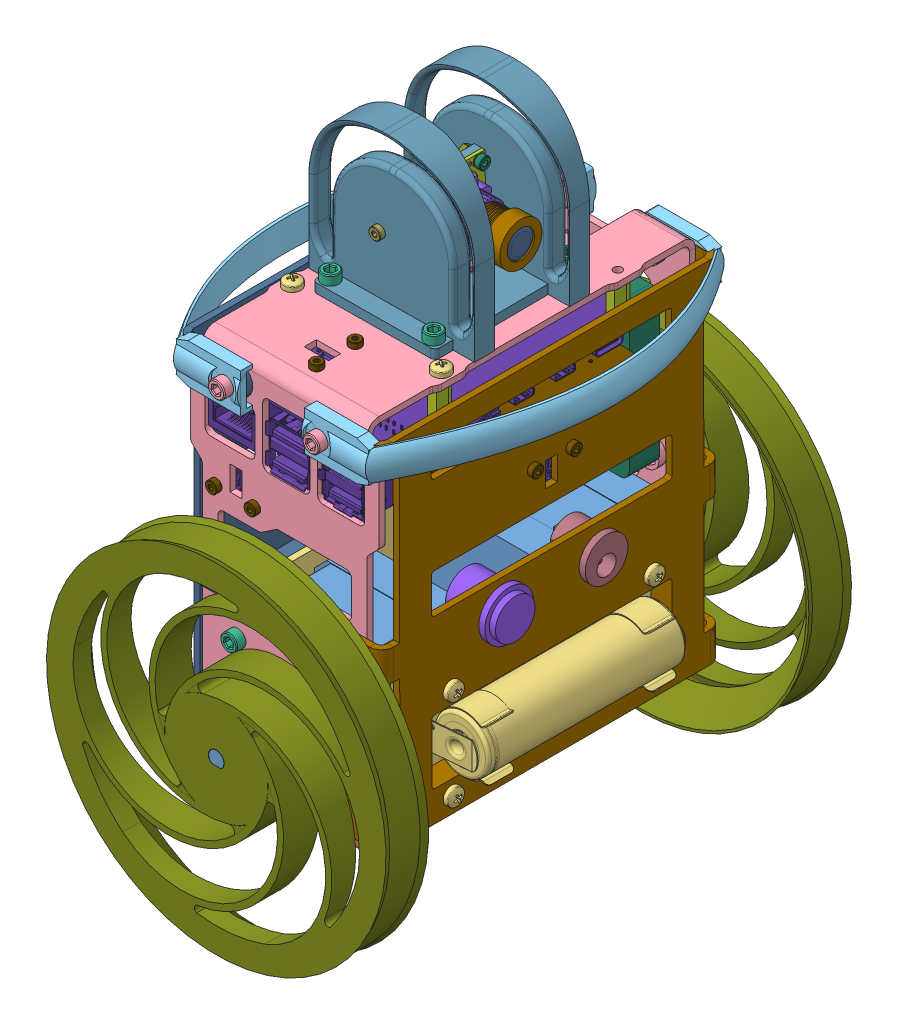
SolidWorks assembly irys5, configuration Domyślna. Lengths in mm.
Overall size (135.28 218.43 153).
149 component instances, 36 part files, 128 mates.
Components (placement in the parent):
- steppermotor-1: steppermotor [Default] at (-42.2578 -7.1789 72.25) size (42.3 42.3 64.5)
- bottomframe_rys3-1: bottomframe_rys3 [Domyślna] at (-43.1924 -31.5373 18.7182) x (0 0 -1) z (0 -1 0) size (108 54 25.86)
- steppermotor-2: steppermotor [Default] at (-42.2578 -7.1789 -31.75) x (-1 0 0) z (0 0 -1) size (42.3 42.3 64.5)
- battery_module-1: battery_module [Domyślna] at (-62.2578 -31.5373 65.25) x (0 0 -1) z (0 -1 0) size (90 40 22.7)
- topframe-1: topframe [Domyślna] at (-44.2495 88.6087 10.8694) x (0 0 -1) z (0 1 0) size (108 62 97.29)
- bumper_front-2: bumper_front [Domyślna] at (-73.7578 82.3211 20.318) x (0 0 -1) z (0 1 0) size (119.34 56.62 18.18)
- bumper_front-3: bumper_front [Domyślna] at (-10.7578 82.314 20.2704) x (0 0 -1) z (0 -1 0) size (119.34 56.62 18.18)
- imu-1: imu [Domyślna] at (-53.5985 -10.4799 25.3181) x (-0.019519 0 -0.999809) z (0 -1 0) size (10.16 22.86 2.23)
- camera_mounted-1: camera_mounted [Domyślna] at (-50.0059 110.2904 17.0046) x (-0.008727 0 -0.999962) z (0.999897 0.011413 -0.008726) size (26.1 24.65 29.88)
  - Camera Module Assem-1: Camera Module Assem [Default] at (-12.4357 -13.5775 -13.0743) size (25 24 24.98)
    - PCB 1-1: PCB 1 [Default] at (8.9736 12.851 19.5114) size (25 24 2.1)
    - Camera Block-1: Camera Block [Default] at (8.9736 15.851 20.5114) size (22 13.5 12.5)
    - Camera end-1: Camera end [Default] at (8.9736 15.851 27.3922) x (0.999924 0.012337 0) z (0 0 1) size (14 14 17.26)
    - Lenz-1: Lenz [Default] at (8.9736 15.851 43.8922) size (9 9 0.5)
    - 15 Pin Ribbon Block Assem-1: 15 Pin Ribbon Block Assem [Default] at (0.7567 20.5462 10.9417) x (1 0 0) z (0 -1 0) size (22 2.5 7)
      - 15 Pin Ribbon Block-1: 15 Pin Ribbon Block [Default] at (8.217 10.8197 14.6952) size (20 2.5 6)
      - Ribbon Clamp-1: Ribbon Clamp [Default] at (8.217 10.8197 14.6952) size (22 2.5 5)
    - 0603 Resistor-1: 0603 Resistor [Default] at (2.3268 23.572 20.4882) size (1.75 0.89 0.66)
    - 0603 Resistor-2: 0603 Resistor [Default] at (4.5768 23.572 20.4882) size (1.75 0.89 0.66)
    - 0603 Resistor-3: 0603 Resistor [Default] at (15.6203 23.5707 20.4857) size (1.75 0.89 0.66)
    - 0603 Resistor-4: 0603 Resistor [Default] at (13.3703 23.5707 20.4857) size (1.75 0.89 0.66)
  - mount-1: mount [Domyślna] at (-15.8432 -12.9016 1.4371) size (25 24 5)
  - M2 x 0.4mm Thread 5mm LONG SOCKET HEAD CAP SCREW-1: M2 x 0.4mm Thread 5mm LONG SOCKET HEAD CAP SCREW [Domyślna] at (7.0379 9.2735 2.5371) x (-0.356462 0.93431 0) z (0 0 -1) size (3.8 3.8 7.09)
  - M2 x 0.4mm Thread 5mm LONG SOCKET HEAD CAP SCREW-2: M2 x 0.4mm Thread 5mm LONG SOCKET HEAD CAP SCREW [Domyślna] at (7.0379 -4.7265 2.5371) x (-0.994039 0.109029 0) z (0 0 -1) size (3.8 3.8 7.09)
  - M2 x 0.4mm Thread 5mm LONG SOCKET HEAD CAP SCREW-3: M2 x 0.4mm Thread 5mm LONG SOCKET HEAD CAP SCREW [Domyślna] at (-13.9621 9.2735 2.5371) x (-0.583934 -0.811801 0) z (0 0 -1) size (3.8 3.8 7.09)
  - M2 x 0.4mm Thread 5mm LONG SOCKET HEAD CAP SCREW-4: M2 x 0.4mm Thread 5mm LONG SOCKET HEAD CAP SCREW [Domyślna] at (-13.9621 -4.7265 2.5371) x (-0.923728 -0.383049 0) z (0 0 -1) size (3.8 3.8 7.09)
  - m2_x_0_4mm_thread_hex_nut-1: m2_x_0_4mm_thread_hex_nut [Domyślna] at (7.0379 9.2735 3.1371) size (4 4.62 1.6)
  - m2_x_0_4mm_thread_hex_nut-2: m2_x_0_4mm_thread_hex_nut [Domyślna] at (7.0379 -4.7265 3.1371) size (4 4.62 1.6)
  - m2_x_0_4mm_thread_hex_nut-3: m2_x_0_4mm_thread_hex_nut [Domyślna] at (-13.9621 -4.7265 3.1371) size (4 4.62 1.6)
  - m2_x_0_4mm_thread_hex_nut-4: m2_x_0_4mm_thread_hex_nut [Domyślna] at (-13.9621 9.2735 3.1371) size (4 4.62 1.6)
- ToF_nut-3: ToF_nut [Domyślna] at (-29.7647 53.9524 20.8423) x (0 1 0) z (1 0 0) size (12.89 18.5 4.22)
  - vl53l1x-1: vl53l1x [Domyślna] at (-6.7913 -9.4823 16.6745) size (12.7 17.78 2.22)
  - m2_x_0_4mm_thread_hex_nut-1: m2_x_0_4mm_thread_hex_nut [Domyślna] at (3.3687 5.7577 15.8745) size (4 4.62 1.6)
  - m2_x_0_4mm_thread_hex_nut-2: m2_x_0_4mm_thread_hex_nut [Domyślna] at (3.3687 -6.9423 15.8745) x (-0.923728 -0.383049 0) z (0 0 -1) size (4 4.62 1.6)
  - m2_x_0_4mm_thread_hex_nut-3: m2_x_0_4mm_thread_hex_nut [Domyślna] at (3.3687 5.7577 18.4945) x (-0.923728 -0.383049 0) z (0 0 -1) size (4 4.62 1.6) (hidden)
  - m2_x_0_4mm_thread_hex_nut-4: m2_x_0_4mm_thread_hex_nut [Domyślna] at (3.3687 -6.9423 18.4945) x (-0.923728 -0.383049 0) z (0 0 -1) size (4 4.62 1.6) (hidden)
- m2_x_0_4mm_thread_6mm_long_sock-3: m2_x_0_4mm_thread_6mm_long_sock [Domyślna] at (-14.4701 57.3211 13.9) x (0 0.924225 0.381849) z (-1 0 0) size (3.8 3.8 8)
- m2_x_0_4mm_thread_6mm_long_sock-5: m2_x_0_4mm_thread_6mm_long_sock [Domyślna] at (-14.4701 57.3211 26.6) x (0 0.924225 0.381849) z (-1 0 0) size (3.8 3.8 8)
- ToF_nut-5: ToF_nut [Domyślna] at (-42.1264 69.3142 59.6577) x (1 0 0) z (0 1 0) size (12.89 18.5 4.22)
  - vl53l1x-1: vl53l1x [Domyślna] at (-6.7913 -9.4823 16.6745) size (12.7 17.78 2.22)
  - m2_x_0_4mm_thread_hex_nut-1: m2_x_0_4mm_thread_hex_nut [Domyślna] at (3.3687 5.7577 15.8745) size (4 4.62 1.6)
  - m2_x_0_4mm_thread_hex_nut-2: m2_x_0_4mm_thread_hex_nut [Domyślna] at (3.3687 -6.9423 15.8745) x (-0.923728 -0.383049 0) z (0 0 -1) size (4 4.62 1.6)
  - m2_x_0_4mm_thread_hex_nut-3: m2_x_0_4mm_thread_hex_nut [Domyślna] at (3.3687 5.7577 18.4945) x (-0.923728 -0.383049 0) z (0 0 -1) size (4 4.62 1.6) (hidden)
  - m2_x_0_4mm_thread_hex_nut-4: m2_x_0_4mm_thread_hex_nut [Domyślna] at (3.3687 -6.9423 18.4945) x (-0.923728 -0.383049 0) z (0 0 -1) size (4 4.62 1.6) (hidden)
- m2_x_0_4mm_thread_6mm_long_sock-7: m2_x_0_4mm_thread_6mm_long_sock [Domyślna] at (-39.3956 84.6087 53.9072) x (-0.868702 0 -0.495335) z (0 -1 0) size (3.8 3.8 8)
- ToF_nut-6: ToF_nut [Domyślna] at (-57.6358 52.0275 52.9555) x (-0.008727 -0.999962 0) z (0 0 1) size (12.89 18.5 4.22)
  - vl53l1x-1: vl53l1x [Domyślna] at (-6.7913 -9.4823 16.6745) size (12.7 17.78 2.22)
  - m2_x_0_4mm_thread_hex_nut-1: m2_x_0_4mm_thread_hex_nut [Domyślna] at (3.3687 5.7577 15.8745) size (4 4.62 1.6)
  - m2_x_0_4mm_thread_hex_nut-2: m2_x_0_4mm_thread_hex_nut [Domyślna] at (3.3687 -6.9423 15.8745) x (-0.923728 -0.383049 0) z (0 0 -1) size (4 4.62 1.6)
  - m2_x_0_4mm_thread_hex_nut-3: m2_x_0_4mm_thread_hex_nut [Domyślna] at (3.3687 5.7577 18.4945) x (-0.923728 -0.383049 0) z (0 0 -1) size (4 4.62 1.6) (hidden)
  - m2_x_0_4mm_thread_hex_nut-4: m2_x_0_4mm_thread_hex_nut [Domyślna] at (3.3687 -6.9423 18.4945) x (-0.923728 -0.383049 0) z (0 0 -1) size (4 4.62 1.6) (hidden)
- ToF_nut-7: ToF_nut [Domyślna] at (-41.6654 54.9524 -12.4555) x (0 1 0) z (0 0 -1) size (12.89 18.5 4.22)
  - vl53l1x-1: vl53l1x [Domyślna] at (-6.7913 -9.4823 16.6745) size (12.7 17.78 2.22)
  - m2_x_0_4mm_thread_hex_nut-1: m2_x_0_4mm_thread_hex_nut [Domyślna] at (3.3687 5.7577 15.8745) size (4 4.62 1.6)
  - m2_x_0_4mm_thread_hex_nut-2: m2_x_0_4mm_thread_hex_nut [Domyślna] at (3.3687 -6.9423 15.8745) x (-0.923728 -0.383049 0) z (0 0 -1) size (4 4.62 1.6)
  - m2_x_0_4mm_thread_hex_nut-3: m2_x_0_4mm_thread_hex_nut [Domyślna] at (3.3687 5.7577 18.4945) x (-0.923728 -0.383049 0) z (0 0 -1) size (4 4.62 1.6) (hidden)
  - m2_x_0_4mm_thread_hex_nut-4: m2_x_0_4mm_thread_hex_nut [Domyślna] at (3.3687 -6.9423 18.4945) x (-0.923728 -0.383049 0) z (0 0 -1) size (4 4.62 1.6) (hidden)
- ToF_nut-9: ToF_nut [Domyślna] at (-54.7508 53.9524 19.6577) x (0 1 0) z (-1 0 0) size (12.89 18.5 4.22)
  - vl53l1x-1: vl53l1x [Domyślna] at (-6.7913 -9.4823 16.6745) size (12.7 17.78 2.22)
  - m2_x_0_4mm_thread_hex_nut-1: m2_x_0_4mm_thread_hex_nut [Domyślna] at (3.3687 5.7577 15.8745) size (4 4.62 1.6)
  - m2_x_0_4mm_thread_hex_nut-2: m2_x_0_4mm_thread_hex_nut [Domyślna] at (3.3687 -6.9423 15.8745) x (-0.923728 -0.383049 0) z (0 0 -1) size (4 4.62 1.6)
  - m2_x_0_4mm_thread_hex_nut-3: m2_x_0_4mm_thread_hex_nut [Domyślna] at (3.3687 5.7577 18.4945) x (-0.923728 -0.383049 0) z (0 0 -1) size (4 4.62 1.6) (hidden)
  - m2_x_0_4mm_thread_hex_nut-4: m2_x_0_4mm_thread_hex_nut [Domyślna] at (3.3687 -6.9423 18.4945) x (-0.923728 -0.383049 0) z (0 0 -1) size (4 4.62 1.6) (hidden)
- m2_x_0_4mm_thread_6mm_long_sock-11: m2_x_0_4mm_thread_6mm_long_sock [Domyślna] at (-70.0322 57.3211 13.9) x (0 -0.924225 -0.381849) z (1 0 0) size (3.8 3.8 8)
- m2_x_0_4mm_thread_6mm_long_sock-12: m2_x_0_4mm_thread_6mm_long_sock [Domyślna] at (-70.0322 57.3211 26.6) x (0 -0.924225 -0.381849) z (1 0 0) size (3.8 3.8 8)
- m2_x_0_4mm_thread_6mm_long_sock-15: m2_x_0_4mm_thread_6mm_long_sock [Domyślna] at (-64.6078 48.6087 68.25) x (-0.262854 -0.964836 0) z (0 0 -1) size (3.8 3.8 8)
- m2_x_0_4mm_thread_6mm_long_sock-16: m2_x_0_4mm_thread_6mm_long_sock [Domyślna] at (-51.9078 48.6087 68.25) x (0.638921 -0.769272 0) z (0 0 -1) size (3.8 3.8 8)
- m2_x_0_4mm_thread_6mm_long_sock-17: m2_x_0_4mm_thread_6mm_long_sock [Domyślna] at (-48.6078 58.3211 -27.75) size (3.8 3.8 8)
- m2_x_0_4mm_thread_6mm_long_sock-18: m2_x_0_4mm_thread_6mm_long_sock [Domyślna] at (-35.9078 58.3211 -27.6076) size (3.8 3.8 8)
- H-H_M3x12mm-1: H-H_M3x12mm [Predeterminado] at (-51.2078 -23.4959 17.65) x (0.837169 0 0.546944) z (0.546944 0 -0.837169) size (5.77 12 5)
- H-H_M3x6mm-1: H-H_M3x6mm [Predeterminado] at (-51.2078 -14.4959 17.65) x (0.837169 0 0.546944) z (0.546944 0 -0.837169) size (5.77 6 5)
- pan cross head_am-2: pan cross head_am [B18.6.7M - M3 x 0.5 x 6 Type I Cross Recessed PHMS --6N] at (-51.2078 -8.0799 17.65) x (0 -1 0) z (0 0 1) size (8.37 5.6 5.6)
- battery_module_H-2: battery_module_H [Domyślna] at (13.655 -6.0808 19.8906) x (0 0 1) z (-1 0 0) size (90 40 24.06)
  - battery_module-1: battery_module [Domyślna] at (-44.6406 -21.0981 81.7004) size (90 40 22.7)
  - H-H_M3x6mm-1: H-H_M3x6mm [Predeterminado] at (-32.6406 13.9019 84.7004) x (1 0 0) z (0 1 0) size (5.77 6 5)
  - H-H_M3x6mm-2: H-H_M3x6mm [Predeterminado] at (33.3594 13.9019 84.7004) x (1 0 0) z (0 1 0) size (5.77 6 5)
  - H-H_M3x6mm-3: H-H_M3x6mm [Predeterminado] at (-32.6406 -16.0981 84.7004) x (1 0 0) z (0 -1 0) size (5.77 6 5)
  - H-H_M3x6mm-4: H-H_M3x6mm [Predeterminado] at (33.3594 -16.0981 84.7004) x (1 0 0) z (0 1 0) size (5.77 6 5)
  - pan cross head_am-1: pan cross head_am [B18.6.7M - M3 x 0.5 x 6 Type I Cross Recessed PHMS --6N] at (-32.6406 -16.0981 77.2589) x (0 0 1) z (-1 0 0) size (8.37 5.6 5.6)
  - pan cross head_am-3: pan cross head_am [B18.6.7M - M3 x 0.5 x 6 Type I Cross Recessed PHMS --6N] at (-32.6406 13.9019 77.2589) x (0 0 1) z (-1 0 0) size (8.37 5.6 5.6)
  - pan cross head_am-4: pan cross head_am [B18.6.7M - M3 x 0.5 x 6 Type I Cross Recessed PHMS --6N] at (33.3594 13.9019 77.2589) x (0 0 1) z (-1 0 0) size (8.37 5.6 5.6)
  - pan cross head_am-5: pan cross head_am [B18.6.7M - M3 x 0.5 x 6 Type I Cross Recessed PHMS --6N] at (33.3594 -16.0981 77.2589) x (0 0 1) z (-1 0 0) size (8.37 5.6 5.6)
- pan cross head_am-3: pan cross head_am [B18.6.7M - M3 x 0.5 x 6 Type I Cross Recessed PHMS --6N] at (-78.4454 -22.1789 53.25) size (8.37 5.6 5.6)
- pan cross head_am-4: pan cross head_am [B18.6.7M - M3 x 0.5 x 6 Type I Cross Recessed PHMS --6N] at (-78.4454 7.8211 53.25) size (8.37 5.6 5.6)
- pan cross head_am-5: pan cross head_am [B18.6.7M - M3 x 0.5 x 6 Type I Cross Recessed PHMS --6N] at (-78.4454 7.8211 -12.75) size (8.37 5.6 5.6)
- pan cross head_am-6: pan cross head_am [B18.6.7M - M3 x 0.5 x 6 Type I Cross Recessed PHMS --6N] at (-78.4454 -22.1789 -12.75) size (8.37 5.6 5.6)
- pan cross head_am-7: pan cross head_am [B18.6.7M - M3 x 0.5 x 6 Type I Cross Recessed PHMS --6N] at (-57.2578 -35.9373 53.25) x (0 1 0) z (0 0 1) size (8.37 5.6 5.6)
- pan cross head_am-8: pan cross head_am [B18.6.7M - M3 x 0.5 x 6 Type I Cross Recessed PHMS --6N] at (-27.2578 -35.9373 53.25) x (0 1 0) z (0 0 1) size (8.37 5.6 5.6)
- pan cross head_am-9: pan cross head_am [B18.6.7M - M3 x 0.5 x 6 Type I Cross Recessed PHMS --6N] at (-57.2578 -35.9373 -12.75) x (0 1 0) z (0 0 1) size (8.37 5.6 5.6)
- pan cross head_am-10: pan cross head_am [B18.6.7M - M3 x 0.5 x 6 Type I Cross Recessed PHMS --6N] at (-27.2578 -35.9373 -12.75) x (0 1 0) z (0 0 1) size (8.37 5.6 5.6)
- battery_module_H-3: battery_module_H [Domyślna] at (-98.1705 -8.277 19.8906) x (0 0 1) z (1 0 0) size (90 40 24.06)
  - battery_module-1: battery_module [Domyślna] at (-44.6406 -21.0981 81.7004) size (90 40 22.7)
  - H-H_M3x6mm-1: H-H_M3x6mm [Predeterminado] at (-32.6406 13.9019 84.7004) x (1 0 0) z (0 1 0) size (5.77 6 5)
  - H-H_M3x6mm-2: H-H_M3x6mm [Predeterminado] at (33.3594 13.9019 84.7004) x (1 0 0) z (0 1 0) size (5.77 6 5)
  - H-H_M3x6mm-3: H-H_M3x6mm [Predeterminado] at (-32.6406 -16.0981 84.7004) x (1 0 0) z (0 -1 0) size (5.77 6 5)
  - H-H_M3x6mm-4: H-H_M3x6mm [Predeterminado] at (33.3594 -16.0981 84.7004) x (1 0 0) z (0 1 0) size (5.77 6 5)
  - pan cross head_am-1: pan cross head_am [B18.6.7M - M3 x 0.5 x 6 Type I Cross Recessed PHMS --6N] at (-32.6406 -16.0981 77.2589) x (0 0 1) z (-1 0 0) size (8.37 5.6 5.6)
  - pan cross head_am-3: pan cross head_am [B18.6.7M - M3 x 0.5 x 6 Type I Cross Recessed PHMS --6N] at (-32.6406 13.9019 77.2589) x (0 0 1) z (-1 0 0) size (8.37 5.6 5.6)
  - pan cross head_am-4: pan cross head_am [B18.6.7M - M3 x 0.5 x 6 Type I Cross Recessed PHMS --6N] at (33.3594 13.9019 77.2589) x (0 0 1) z (-1 0 0) size (8.37 5.6 5.6)
  - pan cross head_am-5: pan cross head_am [B18.6.7M - M3 x 0.5 x 6 Type I Cross Recessed PHMS --6N] at (33.3594 -16.0981 77.2589) x (0 0 1) z (-1 0 0) size (8.37 5.6 5.6)
- pan cross head_am-11: pan cross head_am [B18.6.7M - M3 x 0.5 x 6 Type I Cross Recessed PHMS --6N] at (-6.0701 -22.1789 53.25) x (-1 0 0) z (0 0.924225 0.381849) size (8.37 5.6 5.6)
- pan cross head_am-12: pan cross head_am [B18.6.7M - M3 x 0.5 x 6 Type I Cross Recessed PHMS --6N] at (-6.0701 7.8211 53.25) x (-1 0 0) z (0 0.924225 0.381849) size (8.37 5.6 5.6)
- pan cross head_am-13: pan cross head_am [B18.6.7M - M3 x 0.5 x 6 Type I Cross Recessed PHMS --6N] at (-6.0701 7.8211 -12.75) x (-1 0 0) z (0 0.924225 0.381849) size (8.37 5.6 5.6)
- pan cross head_am-14: pan cross head_am [B18.6.7M - M3 x 0.5 x 6 Type I Cross Recessed PHMS --6N] at (-6.0701 -22.1789 -12.75) x (-1 0 0) z (0 0.924225 0.381849) size (8.37 5.6 5.6)
- M3x6-1: M3x6 [Default] at (-57.7578 82.3211 -40.75) x (0 0 1) z (0.923728 0.383049 0) size (9 5.5 5.5)
- M3x6-2: M3x6 [Default] at (-26.7578 82.3211 -40.75) x (0 0 1) z (0.923728 0.383049 0) size (9 5.5 5.5)
- M3x4-1: M3x4 [Default] at (-26.7578 24.3211 -38.75) x (0 0 1) z (0.923728 0.383049 0) size (7 5.5 5.5)
- M3x4-2: M3x4 [Default] at (-57.7578 24.3211 -38.75) x (0 0 1) z (0.923728 0.383049 0) size (7 5.5 5.5)
- M3x8-1: M3x8 [Default] at (-26.7578 8.3211 -36.75) x (0 0 1) z (0.923728 0.383049 0) size (9 5.5 5.5)
- M3x8-2: M3x8 [Default] at (-57.7578 8.3211 -36.75) x (0 0 1) z (0.923728 0.383049 0) size (9 5.5 5.5)
- M3x8-3: M3x8 [Default] at (-26.7578 -22.6789 -38.75) x (0 0 1) z (-0.923728 -0.383049 0) size (9 5.5 5.5)
- M3x8-4: M3x8 [Default] at (-57.7578 -22.6789 -38.75) x (0 0 1) z (0.923728 0.383049 0) size (9 5.5 5.5)
- M3x6-3: M3x6 [Default] at (-57.7578 82.3211 81.318) x (0 0 -1) z (-0.923728 -0.383049 0) size (9 5.5 5.5)
- M3x6-4: M3x6 [Default] at (-26.7578 82.3211 81.25) x (0 0 -1) z (-0.923728 -0.383049 0) size (9 5.5 5.5)
- M3x4-3: M3x4 [Default] at (-57.7578 24.3211 79.25) x (0 0 -1) z (-0.923728 -0.383049 0) size (7 5.5 5.5)
- M3x4-4: M3x4 [Default] at (-26.7578 24.3211 79.25) x (0 0 -1) z (-0.923728 -0.383049 0) size (7 5.5 5.5)
- M3x8-5: M3x8 [Default] at (-57.7578 8.3211 77.25) x (0 0 -1) z (-0.923728 -0.383049 0) size (9 5.5 5.5)
- M3x8-6: M3x8 [Default] at (-26.7578 8.314 77.25) x (0 0 -1) z (-0.923728 -0.383049 0) size (9 5.5 5.5)
- M3x8-7: M3x8 [Default] at (-57.7578 -22.6789 79.25) x (0 0 -1) z (-0.923728 -0.383049 0) size (9 5.5 5.5)
- M3x8-8: M3x8 [Default] at (-26.7578 -22.6789 79.25) x (0 0 -1) z (-0.923728 -0.383049 0) size (9 5.5 5.5)
- m2_x_0_4mm_thread_6mm_long_sock-19: m2_x_0_4mm_thread_6mm_long_sock [Domyślna] at (-39.3956 84.6087 66.6072) x (-0.868702 0 -0.495335) z (0 -1 0) size (3.8 3.8 8)
- H-M_M3x10x6mm-1: H-M_M3x10x6mm [Predeterminado] at (-66.7578 78.6087 47.25) size (5.77 16 5)
- H-M_M3x10x6mm-2: H-M_M3x10x6mm [Predeterminado] at (-18.2481 78.6087 47.3511) size (5.77 16 5)
- H-M_M3x10x6mm-5: H-M_M3x10x6mm [Predeterminado] at (-66.7578 78.6087 -10.7875) size (5.77 16 5)
- H-M_M3x10x6mm-6: H-M_M3x10x6mm [Predeterminado] at (-17.7578 78.6087 -10.75) size (5.77 16 5)
- pan cross head_am-15: pan cross head_am [B18.6.7M - M3 x 0.5 x 6 Type I Cross Recessed PHMS --6N] at (-66.7578 93.0087 47.25) x (0 -1 0) z (-0.546944 0 0.837169) size (8.37 5.6 5.6)
- pan cross head_am-16: pan cross head_am [B18.6.7M - M3 x 0.5 x 6 Type I Cross Recessed PHMS --6N] at (-17.7578 93.0087 -10.75) x (0 -1 0) z (-0.546944 0 0.837169) size (8.37 5.6 5.6) (hidden)
- pan cross head_am-17: pan cross head_am [B18.6.7M - M3 x 0.5 x 6 Type I Cross Recessed PHMS --6N] at (-66.7578 93.0087 -10.75) x (0 -1 0) z (-0.546944 0 0.837169) size (8.37 5.6 5.6)
- pan cross head_am-18: pan cross head_am [B18.6.7M - M3 x 0.5 x 6 Type I Cross Recessed PHMS --6N] at (-17.7578 93.0087 47.25) x (0 -1 0) z (-0.546944 0 0.837169) size (8.37 5.6 5.6)
- switch_simple-1: switch_simple [Domyślna] at (-4.4701 21.3211 36.25) x (0 0 1) z (-1 0 0) size (16 16 16)
- front-4: front [Domyślna] at (-10.5869 69.5154 20.4189) x (0 0 -1) z (0.002583 -0.999997 0) size (112 23.29 115)
- back-1: back [Domyślna] at (-74.0454 69.4652 20.0764) x (0 0 1) z (0 -1 0) size (112 23.29 115)
- 430250200.stp-4: 430250200.stp [Domyślna] at (-25.0029 52.3587 -6.87) x (-1 0 0) z (0 0 -1) size (5.28 14 10.85)
- 430250200.stp-5: 430250200.stp [Domyślna] at (-40.3546 52.3587 -6.985) x (-1 0 0) z (0 0 -1) size (5.28 14 10.85)
- 430250200.stp-6: 430250200.stp [Domyślna] at (-47.7558 52.3587 -6.985) x (-1 0 0) z (0 0 -1) size (5.28 14 10.85)
- 430250200.stp-7: 430250200.stp [Domyślna] at (-31.8443 52.3587 -6.985) x (-1 0 0) z (0 0 -1) size (5.28 14 10.85)
- M2 x 0.4mm Thread 10mm LONG SOCKET HEAD CAP SCREW-5: M2 x 0.4mm Thread 10mm LONG SOCKET HEAD CAP SCREW [Domyślna] at (-46.1456 112.6087 11.197) x (-0.266178 0.963921 0.002323) z (0.008727 0 0.999962) size (3.8 3.8 12.09)
- M2 x 0.4mm Thread 10mm LONG SOCKET HEAD CAP SCREW-6: M2 x 0.4mm Thread 10mm LONG SOCKET HEAD CAP SCREW [Domyślna] at (-45.9885 112.6087 29.1949) x (-0.999897 -0.011413 0.008726) z (-0.008727 0 -0.999962) size (3.8 3.8 12.09)
- M3x8-9: M3x8 [Default] at (-25.2578 96.6087 -1.75) x (0 -1 0) z (-0.923728 0 0.383049) size (9 5.5 5.5)
- M3x8-13: M3x8 [Default] at (-59.2578 96.6087 42.25) x (0 -1 0) z (-0.923728 0 0.383049) size (9 5.5 5.5)
- M3x8-14: M3x8 [Default] at (-25.2578 96.6087 42.25) x (0 -1 0) z (-0.923728 0 0.383049) size (9 5.5 5.5)
- M3x8-15: M3x8 [Default] at (-59.2578 96.6087 -1.75) x (0 -1 0) z (-0.923728 0 0.383049) size (9 5.5 5.5)
- Panel_Mount_2mm_Power_Plug_v2.step-1: Panel_Mount_2mm_Power_Plug_v2.step [Domyślna] at (-6.4559 21.3664 4.25) x (0 -0.000012 -1) z (-0.002583 0.999997 -0.000012) size (14 13.69 14)
- mount3-1: mount3 [Domyślna] at (-42.0651 90.6087 20.3975) x (-0.008727 0 -0.999962) z (0.999962 0 -0.008727) size (50 53 54.12)
- fan_simple_50x50-1: fan_simple_50x50 [Domyślna] at (-42.2578 53.8211 -24.0253) x (1 0 0) z (0 -1 0) size (50 10 50)
- Wheel_new-1: Wheel_new [Domyślna] at (15.96 7.3364 76.75) x (-0.241922 0.970296 0) z (0 0 1) size (111.6 111.6 20)
- Wheel_new-2: Wheel_new [Domyślna] at (-100.4755 7.3364 -36.25) x (0.241922 0.970296 0) z (0 0 -1) size (111.6 111.6 20)
- Raspberry Pi 4 Model B-2: Raspberry Pi 4 Model B [Default] at (-42.2578 77.8087 28.25) x (0 0 1) z (1 0 0) size (88.99 19.91 58.4)
- rys_board_v4.1-1: rys_board_v4.1 [Domyślna] at (-94.2277 65.9587 -55.6601) x (1 0 0) z (0 -1 0) size (56.3 64 18.7)
Mates (geometry in assembly coordinates):
- Koncentryczne1: concentric aligned: cylinder of steppermotor-1 through (-26.7578 -22.6789 64.75) axis (0 0 1) radius 1.25; cylinder of bottomframe_rys3-1 through (-26.7578 -22.6789 74.25) axis (0 0 1) radius 1.6
- Koncentryczne2: concentric aligned: cylinder of steppermotor-1 through (-57.7578 -22.6789 64.75) axis (0 0 1) radius 1.25; cylinder of bottomframe_rys3-1 through (-57.7578 -22.6789 74.25) axis (0 0 1) radius 1.6
- Wspólnie1: coincident anti-aligned: plane of steppermotor-1 through (-64.2538 -29.1749 72.25) normal (0 0 1); plane of bottomframe_rys3-1 through (-42.2578 -7.6789 72.25) normal (0 0 -1)
- Koncentryczne3: concentric aligned: cylinder of bottomframe_rys3-1 through (-57.7578 -22.6789 -33.75) axis (0 0 -1) radius 1.6; cylinder of steppermotor-2 through (-57.7578 -22.6789 -24.25) axis (0 0 -1) radius 1.25
- Koncentryczne4: concentric aligned: circle of bottomframe_rys3-1; cylinder of steppermotor-2 through (-26.7578 -22.6789 -24.25) axis (0 0 -1) radius 1.25
- Wspólnie2: coincident anti-aligned: plane of bottomframe_rys3-1 through (-42.2578 -161.6789 -31.75) normal (0 0 1); plane of steppermotor-2 through (-20.2618 -29.1749 -31.75) normal (0 0 -1)
- Koncentryczne7: concentric aligned: cylinder of steppermotor-2 through (-26.7578 8.3211 -24.25) axis (0 0 -1) radius 1.25; cylinder of topframe-1 through (-26.7578 8.3211 -33.75) axis (0 0 -1) radius 1.6
- Koncentryczne8: concentric aligned: cylinder of steppermotor-1 through (-57.7578 8.3211 64.75) axis (0 0 1) radius 1.25; cylinder of topframe-1 through (-57.7578 8.3211 74.25) axis (0 0 1) radius 1.6
- Wspólnie4: coincident anti-aligned: plane of steppermotor-1 through (-64.2538 -29.1749 72.25) normal (0 0 1); plane of topframe-1 through (-71.2578 51.9927 72.25) normal (0 0 -1)
- Koncentryczne18: concentric aligned: cylinder of bottomframe_rys3-1 through (-26.7578 -22.6789 -33.75) axis (0 0 -1) radius 1.6; cylinder of steppermotor-2 through (-26.7578 -22.6789 -24.25) axis (0 0 -1) radius 1.25
- Koncentryczne55: concentric aligned: cylinder of battery_module-1 through (-51.2078 -29.4959 17.65) axis (0 1 0) radius 1.1; cylinder of imu-1 through (-51.2078 -11.4959 17.65) axis (0 1 0) radius 1.0922
- Koncentryczne56: concentric anti-aligned: cylinder of bottomframe_rys3-1 through (-27.2578 -33.5373 53.25) axis (0 -1 0) radius 1.4; cylinder of battery_module-1 through (-27.2578 -29.4959 53.25) axis (0 1 0) radius 1.6
- Koncentryczne57: concentric anti-aligned: cylinder of bottomframe_rys3-1 through (-57.2578 -33.5373 -12.75) axis (0 -1 0) radius 1.4; cylinder of battery_module-1 through (-57.2578 -29.4959 -12.75) axis (0 1 0) radius 1.6
- Wspólnie27: coincident anti-aligned: plane of bottomframe_rys3-1 through (-42.2578 -31.5373 97.25) normal (0 1 0); plane of battery_module-1 through (-62.2578 -31.5373 65.25) normal (0 -1 0)
- Wspólnie61: coincident anti-aligned: plane of topframe-1 through (-71.2578 88.6087 109.5784) normal (0 -1 0); plane of ToF_nut-5/m2_x_0_4mm_thread_hex_nut-4 through (-37.3526 88.6087 64.7673) normal (0 1 0)
- Koncentryczne104: concentric aligned: cylinder of topframe-1 through (-39.3956 90.6087 53.9072) axis (0 1 0) radius 1.25; cylinder of m2_x_0_4mm_thread_6mm_long_sock-7 through (-39.3956 92.6087 53.9072) axis (0 1 0) radius 1.9
- Wspólnie65: coincident anti-aligned: plane of topframe-1 through (-71.2578 90.6087 109.5784) normal (0 1 0); plane of m2_x_0_4mm_thread_6mm_long_sock-7 through (-39.3956 90.6087 53.9072) normal (0 -1 0)
- Wspólnie67: coincident anti-aligned: plane of topframe-1 through (-71.2578 51.9927 72.25) normal (0 0 -1); plane of ToF_nut-6/m2_x_0_4mm_thread_hex_nut-4 through (-62.7869 47.2984 72.25) normal (0 0 1)
- Wspólnie68: coincident anti-aligned: plane of topframe-1 through (-71.2578 230.6495 -31.75) normal (0 0 1); plane of ToF_nut-7/m2_x_0_4mm_thread_hex_nut-3 through (-34.075 59.7262 -31.75) normal (0 0 -1)
- Wspólnie78: coincident anti-aligned: plane of topframe-1 through (-71.2578 51.9927 74.25) normal (0 0 1); plane of m2_x_0_4mm_thread_6mm_long_sock-15 through (-64.6078 48.6087 74.25) normal (0 0 -1)
- Wspólnie79: coincident anti-aligned: plane of topframe-1 through (-71.2578 51.9927 74.25) normal (0 0 1); plane of m2_x_0_4mm_thread_6mm_long_sock-16 through (-51.9078 48.6087 74.25) normal (0 0 -1)
- Wspólnie80: coincident anti-aligned: plane of topframe-1 through (-71.2578 230.6495 -33.75) normal (0 0 -1); plane of m2_x_0_4mm_thread_6mm_long_sock-17 through (-48.6078 58.3211 -33.75) normal (0 0 1)
- Koncentryczne125: concentric aligned: cylinder of battery_module-1 through (-51.2078 -29.4959 17.65) axis (0 1 0) radius 1.1; cylinder of H-H_M3x12mm-1 through (-51.2078 -29.4959 17.65) axis (0 1 0) radius 1.5
- Wspólnie82: coincident anti-aligned: plane of battery_module-1 through (-62.2578 -29.4959 65.25) normal (0 1 0); plane of H-H_M3x12mm-1 through (-51.2078 -29.4959 17.65) normal (0 -1 0)
- Wspólnie83: coincident anti-aligned: circle of H-H_M3x12mm-1; cylinder of H-H_M3x6mm-1 through (-51.2078 -17.4959 17.65) axis (0 1 0) radius 1.5
- Wspólnie84: coincident anti-aligned: plane of H-H_M3x12mm-1 through (-51.2078 -17.4959 17.65) normal (0 1 0); plane of H-H_M3x6mm-1 through (-51.2078 -17.4959 17.65) normal (0 -1 0)
- Wspólnie85: coincident anti-aligned: plane of imu-1 through (-53.5985 -11.4959 25.3181) normal (0 -1 0); plane of H-H_M3x6mm-1 through (-51.2078 -11.4959 17.65) normal (0 1 0)
- Koncentryczne1261: concentric aligned: cylinder of imu-1 through (-51.2078 -11.4959 17.65) axis (0 1 0) radius 1.0922; cylinder of pan cross head_am-2 through (-51.2078 17.3201 17.65) axis (0 1 0) radius 2.8
- Wspólnie871: coincident anti-aligned: plane of imu-1 through (-53.5985 -10.4799 25.3181) normal (0 1 0); plane of pan cross head_am-2 through (-49.7078 -10.4799 17.65) normal (0 -1 0)
- Koncentryczne1331: concentric aligned: cylinder of bottomframe_rys3-1 through (-57.2578 -33.5373 53.25) axis (0 -1 0) radius 1.4; cylinder of pan cross head_am-7 through (-57.2578 -61.3373 53.25) axis (0 -1 0) radius 2.8
- Wspólnie931: coincident anti-aligned: plane of bottomframe_rys3-1 through (-42.2578 -33.5373 97.25) normal (0 -1 0); plane of pan cross head_am-7 through (-58.7578 -33.5373 53.25) normal (0 1 0)
- Koncentryczne1341: concentric aligned: cylinder of bottomframe_rys3-1 through (-27.2578 -33.5373 53.25) axis (0 -1 0) radius 1.4; cylinder of pan cross head_am-8 through (-27.2578 -61.3373 53.25) axis (0 -1 0) radius 2.8
- Wspólnie941: coincident anti-aligned: plane of bottomframe_rys3-1 through (-42.2578 -33.5373 97.25) normal (0 -1 0); plane of pan cross head_am-8 through (-28.7578 -33.5373 53.25) normal (0 1 0)
- Koncentryczne1351: concentric aligned: cylinder of bottomframe_rys3-1 through (-57.2578 -33.5373 -12.75) axis (0 -1 0) radius 1.4; cylinder of pan cross head_am-9 through (-57.2578 -61.3373 -12.75) axis (0 -1 0) radius 2.8
- Wspólnie951: coincident anti-aligned: plane of bottomframe_rys3-1 through (-42.2578 -33.5373 97.25) normal (0 -1 0); plane of pan cross head_am-9 through (-58.7578 -33.5373 -12.75) normal (0 1 0)
- Koncentryczne1361: concentric aligned: cylinder of bottomframe_rys3-1 through (-27.2578 -33.5373 -12.75) axis (0 -1 0) radius 1.4; cylinder of pan cross head_am-10 through (-27.2578 -61.3373 -12.75) axis (0 -1 0) radius 2.8
- Wspólnie961: coincident anti-aligned: plane of bottomframe_rys3-1 through (-42.2578 -33.5373 97.25) normal (0 -1 0); plane of pan cross head_am-10 through (-28.7578 -33.5373 -12.75) normal (0 1 0)
- Koncentryczne148: concentric aligned: cylinder of topframe-1 through (-26.7578 8.3211 -33.75) axis (0 0 -1) radius 1.6; cylinder of M3x8-1 through (-26.7578 8.3211 -125.4555) axis (0 0 -1) radius 2.75
- Wspólnie107: coincident anti-aligned: plane of topframe-1 through (-71.2578 230.6495 -33.75) normal (0 0 -1); plane of M3x8-1 through (-26.187 6.9447 -33.75) normal (0 0 1)
- Koncentryczne149: concentric aligned: cylinder of topframe-1 through (-57.7578 8.3211 -33.75) axis (0 0 -1) radius 1.6; cylinder of M3x8-2 through (-57.7578 8.3211 -125.4555) axis (0 0 -1) radius 2.75
- Wspólnie108: coincident anti-aligned: plane of topframe-1 through (-71.2578 230.6495 -33.75) normal (0 0 -1); plane of M3x8-2 through (-57.187 6.9447 -33.75) normal (0 0 1)
- Koncentryczne150: concentric aligned: cylinder of bottomframe_rys3-1 through (-57.7578 -22.6789 -33.75) axis (0 0 -1) radius 1.6; cylinder of M3x8-4 through (-57.7578 -22.6789 -127.4555) axis (0 0 -1) radius 2.75
- Koncentryczne153: concentric aligned: circle of topframe-1; cylinder of M3x6-3 through (-57.7578 82.3211 170.0235) axis (0 0 1) radius 2.75
- Koncentryczne155: concentric aligned: cylinder of topframe-1 through (-57.7578 24.3211 74.25) axis (0 0 1) radius 1.6; cylinder of M3x4-3 through (-57.7578 24.3211 167.9555) axis (0 0 1) radius 2.75
- Koncentryczne158: concentric aligned: cylinder of topframe-1 through (-26.7578 8.314 74.25) axis (0 0 1) radius 1.6; cylinder of M3x8-6 through (-26.7578 8.314 165.9555) axis (0 0 1) radius 2.75
- Koncentryczne159: concentric aligned: cylinder of topframe-1 through (-57.7578 8.3211 74.25) axis (0 0 1) radius 1.6; cylinder of M3x8-5 through (-57.7578 8.3211 165.9555) axis (0 0 1) radius 2.75
- Wspólnie115: coincident anti-aligned: plane of topframe-1 through (-71.2578 51.9927 74.25) normal (0 0 1); plane of M3x8-5 through (-57.187 6.9447 74.25) normal (0 0 -1)
- Wspólnie116: coincident anti-aligned: plane of topframe-1 through (-71.2578 51.9927 74.25) normal (0 0 1); plane of M3x8-6 through (-26.187 6.9376 74.25) normal (0 0 -1)
- Równolegle1: parallel aligned: plane of ToF_nut-7/m2_x_0_4mm_thread_hex_nut-1 through (-34.7531 56.3211 -27.53) normal (0 0 1); plane of m2_x_0_4mm_thread_6mm_long_sock-18 through (-35.9078 58.3211 -33.6076) normal (0 0 1)
- Koncentryczne1462: concentric aligned: circle of topframe-1; circle of m2_x_0_4mm_thread_6mm_long_sock-19
- Koncentryczne1463: concentric anti-aligned: circle of bumper2-1; circle of M3x6-7
- Wspólnie970: coincident anti-aligned: plane of bumper2-1 through (-6.0454 102.864 47.0753) normal (1 0 0); plane of M3x6-7 through (-6.0454 81.4447 41.6793) normal (-1 0 0)
- Koncentryczne1464: concentric anti-aligned: circle of bumper2-2; circle of M3x6-8
- Wspólnie971: coincident anti-aligned: plane of bumper2-2 through (-6.0454 102.864 3.0753) normal (1 0 0); plane of M3x6-8 through (-6.0454 81.4447 -2.3207) normal (-1 0 0)
- Koncentryczne1465: concentric aligned: circle of bumper2-1; circle of M3x6-6
- Koncentryczne1466: concentric aligned: circle of bumper2-2; circle of M3x6-5
- Koncentryczne1483: concentric aligned: circle of H-M_M3x10x6mm-1; circle of rys_PCB_rpi_simple-2
- Wspólnie978: coincident anti-aligned: plane of H-M_M3x10x6mm-1 through (-66.7578 78.6087 47.25) normal (0 -1 0); plane of rys_PCB_rpi_simple-2 through (-42.2266 78.6087 28.4747) normal (0 1 0)
- Koncentryczne1484: concentric aligned: circle of H-M_M3x10x6mm-2; circle of rys_PCB_rpi_simple-2
- Wspólnie979: coincident anti-aligned: plane of H-M_M3x10x6mm-2; plane of rys_PCB_rpi_simple-2 through (-42.2266 78.6087 28.4747) normal (0 1 0)
- Koncentryczne1485: concentric aligned: circle of H-M_M3x10x6mm-5; circle of rys_PCB_rpi_simple-2
- Wspólnie980: coincident anti-aligned: plane of H-M_M3x10x6mm-5 through (-66.7578 78.6087 -10.7875) normal (0 -1 0); plane of rys_PCB_rpi_simple-2 through (-42.2266 78.6087 28.4747) normal (0 1 0)
- Koncentryczne1486: concentric aligned: circle of H-M_M3x10x6mm-6; circle of rys_PCB_rpi_simple-2
- Wspólnie981: coincident anti-aligned: plane of H-M_M3x10x6mm-6 through (-17.7578 78.6087 -10.75) normal (0 -1 0); plane of rys_PCB_rpi_simple-2 through (-42.2266 78.6087 28.4747) normal (0 1 0)
- Koncentryczne1487: concentric anti-aligned: circle of topframe-1; circle of H-M_M3x10x6mm-1
- Wspólnie982: coincident anti-aligned: plane of topframe-1 through (-71.2578 88.6087 109.5784) normal (0 -1 0); plane of H-M_M3x10x6mm-1 through (-66.7578 88.6087 47.25) normal (0 1 0)
- Koncentryczne1490: concentric aligned: circle of topframe-1; circle of M3X6_PLASTIC-2
- Wspólnie983: coincident aligned: plane of topframe-1 through (-71.2578 90.6087 109.5784) normal (0 1 0); circle of M3X6_PLASTIC-2
- Koncentryczne1491: concentric aligned: circle of topframe-1; circle of M3X6_PLASTIC-3
- Wspólnie985: coincident aligned: plane of topframe-1 through (-71.2578 90.6087 109.5784) normal (0 1 0); circle of M3X6_PLASTIC-3
- Koncentryczne1492: concentric aligned: circle of topframe-1; circle of M3X6_PLASTIC-1
- Wspólnie986: coincident aligned: plane of topframe-1 through (-71.2578 90.6087 109.5784) normal (0 1 0); circle of M3X6_PLASTIC-1
- Koncentryczne1493: concentric aligned: circle of topframe-1; circle of M3X6_PLASTIC-4
- Wspólnie987: coincident aligned: plane of topframe-1 through (-71.2578 90.6087 109.5784) normal (0 1 0); circle of M3X6_PLASTIC-4
- Stycznie1: tangent: circle of topframe-1; circle of front-4
- Koncentryczne1502: concentric aligned: circle of topframe-1; circle of front-4
- Koncentryczne1506: concentric aligned: circle of bottomframe_rys3-1; circle of frontv2-1
- Koncentryczne1507: concentric aligned: circle of topframe-1; circle of frontv2-1
- Wspólnie1015: coincident anti-aligned: plane of topframe-1 through (-71.2578 90.6087 109.5784) normal (0 1 0); plane of m2_x_0_4mm_thread_6mm_long_sock-19 through (-39.3956 90.6087 66.6072) normal (0 -1 0)
- Równolegle8: parallel anti-aligned: plane of rys_PCB_rpi_simple-2 through (-27.3114 55.3587 -4.0403) normal (0 -1 0); plane of 430250200.stp-4 through (-26.9279 56.0087 -3.44) normal (0 1 0)
- Wspólnie1024: coincident anti-aligned: plane of rys_PCB_rpi_simple-2 through (-50.9865 55.3587 -4.0153) normal (0 -1 0); plane of 430250200.stp-6 through (-49.6808 56.0087 -3.555) normal (0 1 0)
- Wspólnie1025: coincident anti-aligned: plane of rys_PCB_rpi_simple-2 through (-43.1115 55.3587 -4.0153) normal (0 -1 0); plane of 430250200.stp-5 through (-42.2796 56.0087 -3.555) normal (0 1 0)
- Wspólnie1026: coincident anti-aligned: plane of rys_PCB_rpi_simple-2 through (-35.2115 55.3587 -4.0153) normal (0 -1 0); plane of 430250200.stp-7 through (-33.7693 56.0087 -3.555) normal (0 1 0)
- Koncentryczne1524: concentric aligned: circle of mount2-1; circle of M3x8-13
- Wspólnie1031: coincident anti-aligned: plane of mount2-1 through (-60.7578 93.6087 -3.25) normal (0 1 0); plane of M3x8-13 through (-58.687 93.6087 43.6264) normal (0 -1 0)
- Koncentryczne1525: concentric aligned: circle of mount2-1; circle of M3x8-14
- Koncentryczne1526: concentric aligned: circle of mount2-1; circle of M3x8-15
- Koncentryczne1527: concentric aligned: circle of mount2-1; circle of M3x8-9
- Wspólnie1032: coincident aligned: plane of mount2-1 through (-60.7578 93.6087 -3.25) normal (0 1 0); circle of M3x8-14
- Wspólnie1033: coincident aligned: plane of mount2-1 through (-60.7578 93.6087 -3.25) normal (0 1 0); circle of M3x8-15
- Wspólnie1034: coincident anti-aligned: plane of mount2-1 through (-60.7578 93.6087 -3.25) normal (0 1 0); plane of M3x8-9 through (-24.687 93.6087 -0.3736) normal (0 -1 0)
- Koncentryczne1531: concentric anti-aligned: circle of mount2-1; circle of M2 x 0.4mm Thread 10mm LONG SOCKET HEAD CAP SCREW-6
- Wspólnie1036: coincident anti-aligned: plane of mount2-1 through (-42.2578 133.6087 39.25) normal (0 0 1); plane of M2 x 0.4mm Thread 10mm LONG SOCKET HEAD CAP SCREW-6 through (-45.9012 112.6087 39.1945) normal (-0.008727 0 -0.999962)
- Koncentryczne1533: concentric aligned: circle of mount2-1; circle of M2 x 0.4mm Thread 10mm LONG SOCKET HEAD CAP SCREW-5
- Wspólnie1038: coincident anti-aligned: plane of mount2-1 through (-42.2578 133.6087 1.25) normal (0 0 -1); plane of M2 x 0.4mm Thread 10mm LONG SOCKET HEAD CAP SCREW-5 through (-46.2328 112.6087 1.1974) normal (0.008727 0 0.999962)
- Koncentryczne1534: concentric anti-aligned: circle of front-4; circle of Panel_Mount_2mm_Power_Plug_v2.step-1
- Wspólnie1040: coincident anti-aligned: plane of frontv5-4 through (-8.62 82.361 91.25) normal (0.999997 0.002583 0); circle of Panel_Mount_2mm_Power_Plug_v2.step-1
- Koncentryczne1535: concentric aligned: circle of M3x8-9; circle of mount3-1
- Wspólnie1051: coincident anti-aligned: plane of topframe-1 through (-71.2578 90.6087 109.5784) normal (0 1 0); plane of mount3-1 through (-60.7695 90.6087 -2.9402) normal (0 -1 0)
- Koncentryczne1539: concentric aligned: circle of M2 x 0.4mm Thread 10mm LONG SOCKET HEAD CAP SCREW-6; circle of mount3-1
- Koncentryczne1540: concentric anti-aligned: circle of M2 x 0.4mm Thread 10mm LONG SOCKET HEAD CAP SCREW-5; circle of mount3-1
- Wspólnie1053: coincident aligned: circle of camera_mounted-1/mount-1; circle of mount3-1
- Koncentryczne1541: concentric anti-aligned: circle of topframe-1; circle of m2_x_0_4mm_thread_6mm_long_sock-18
- Koncentryczne1542: concentric anti-aligned: circle of topframe-1; circle of m2_x_0_4mm_thread_6mm_long_sock-17
- Koncentryczne1543: concentric aligned: circle of ToF_nut-7/vl53l1x-1; circle of m2_x_0_4mm_thread_6mm_long_sock-17
- Koncentryczne1544: concentric anti-aligned: circle of topframe-1; circle of fan_simple_50x50-1
- Wspólnie1055: coincident anti-aligned: plane of rys_PCB_rpi_simple-2 through (-14.2266 78.6087 -14.0253) normal (0 0 -1); plane of fan_simple_50x50-1 through (-64.2578 31.8211 -14.0253) normal (0 0 1)
- Koncentryczne1545: concentric aligned: circle of steppermotor-1; circle of Wheel_new-1
- Wspólnie1061: coincident aligned: plane of steppermotor-1 through (-44.8633 -9.2845 96.75) normal (0 0 1); plane of Wheel_new-1 through (-28.7585 -61.3214 96.75) normal (0 0 1)
- Koncentryczne1547: concentric aligned: circle of steppermotor-2; circle of Wheel_new-2
- Wspólnie1062: coincident aligned: plane of steppermotor-2 through (-39.6522 -9.2845 -56.25) normal (0 0 -1); plane of Wheel_new-2 through (-55.757 -61.3214 -56.25) normal (0 0 -1)
- Koncentryczne1548: concentric aligned: circle of topframe-1; circle of ToF_nut-6/m2_x_0_4mm_thread_hex_nut-3
- Koncentryczne1549: concentric aligned: circle of topframe-1; circle of m2_x_0_4mm_thread_6mm_long_sock-15
- Koncentryczne1550: concentric aligned: circle of topframe-1; circle of m2_x_0_4mm_thread_6mm_long_sock-16
- Koncentryczne1554: concentric aligned: circle of topframe-1; circle of bumper_front-3
- Koncentryczne1555: concentric anti-aligned: circle of topframe-1; circle of bumper_front-2
- Koncentryczne1556: concentric anti-aligned: circle of H-M_M3x10x6mm-1; circle of Raspberry Pi 4 Model B-2
- Koncentryczne1559: concentric aligned: circle of topframe-1; circle of pan cross head_am-16
- Koncentryczne1560: concentric aligned: circle of topframe-1; circle of H-M_M3x10x6mm-6
- Koncentryczne1561: concentric aligned: circle of H-M_M3x10x6mm-6; circle of Raspberry Pi 4 Model B-2
- Wspólnie1066: coincident anti-aligned: plane of topframe-1 through (-71.2578 88.6087 109.5784) normal (0 -1 0); plane of H-M_M3x10x6mm-2 through (-18.2481 88.6087 47.3511) normal (0 1 0)
- Wspólnie1067: coincident anti-aligned: plane of H-M_M3x10x6mm-2 through (-18.2481 78.6087 47.3511) normal (0 -1 0); plane of Raspberry Pi 4 Model B-2 through (-42.2578 78.6087 28.25) normal (0 1 0)
- Wspólnie1075: coincident aligned: line of Raspberry Pi 4 Model B-2 through (-68.3478 74.5087 -5.56) axis (0 0 -1); line of rys_board_v4.1-1 through (-68.3478 74.5087 -5.2) axis (0 0 -1)
- Wspólnie1076: coincident aligned: line of Raspberry Pi 4 Model B-2 through (-68.3478 74.5087 -6.2) axis (1 0 0); line of rys_board_v4.1-1 through (-68.3478 74.5087 -6.2) axis (1 0 0)
- Wspólnie1078: coincident aligned: line of 430250200.stp-4 through (-26.2029 56.0087 -4.17) axis (1 0 0); line of rys_board_v4.1-1 through (-24.6976 56.0087 -4.17) axis (1 0 0)
- Wspólnie1079: coincident aligned: line of 430250200.stp-7 through (-30.6443 56.0087 -9.685) axis (-1 0 0); line of rys_board_v4.1-1 through (-30.0576 56.0087 -9.685) axis (-1 0 0)
- Wspólnie1080: coincident aligned: line of 430250200.stp-5 through (-39.1546 56.0087 -6.685) axis (-1 0 0); line of rys_board_v4.1-1 through (-37.9576 56.0087 -6.685) axis (-1 0 0)
- Wspólnie1081: coincident aligned: line of 430250200.stp-6 through (-46.5558 56.0087 -9.685) axis (-1 0 0); line of rys_board_v4.1-1 through (-45.8326 56.0087 -9.685) axis (-1 0 0)
